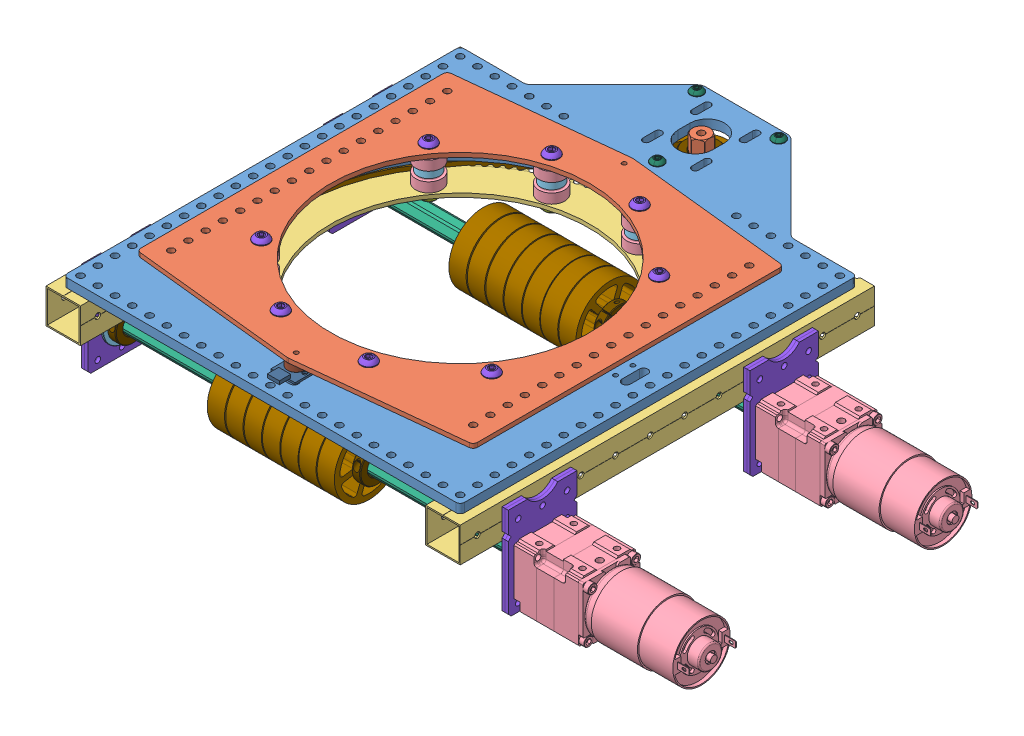
SolidWorks assembly WCP-0280 Rev1 - GreyT Turret, configuration Default. Lengths in mm.
Overall size (454.1 179.88 363.61).
150 component instances, 27 part files, 4 mates.
Components (placement in the parent):
- WCP-0280-001 Rev1-1: WCP-0280-001 Rev1 [Default] at origin size (292.1 6.6 356.64)
- spinner_tray_+_sprocket^WCP-0280 Rev1 - GreyT Turret-1: spinner_tray_+_sprocket^WCP-0280 Rev1 - GreyT Turret [Default] at origin size (248.55 39.23 334.09)
  - WCP-0280-002 Rev1-1: WCP-0280-002 Rev1 [Default] at (0 12.9476 0) size (247.65 3.17 254)
  - WCP-0280-004 Rev1-1: WCP-0280-004 Rev1 [Default] at (0 -14.1605 0) size (246.3 3.25 246.3)
  - bearing_assembly^spinner_tray_+_sprocket-1: bearing_assembly^spinner_tray_+_sprocket [Default] at (-31.5529 25.185 -41.3287) size (26.53 39.23 26.53)
    - WCP-0212_0_250_radial_bearing-1: WCP-0212_0_250_radial_bearing [Default] at (-53.2118 -18.2653 102.9139) x (-0.999427 0 0.033839) z (0 -1 0) size (19.05 19.05 7.14)
    - WCP-0212_0_250_radial_bearing-2: WCP-0212_0_250_radial_bearing [Default] at (-53.2118 -32.1147 102.9139) x (-0.572891 0 0.819632) z (0 1 0) size (19.05 19.05 7.14)
    - WCP-0041_0_250_radial_bearing-1: WCP-0041_0_250_radial_bearing [Default] at (-53.2118 -25.19 102.9139) x (-0.872331 0 0.488916) z (0 -1 0) size (15.88 15.88 4.98)
    - NFS-0011_0_250ID_fiber_washer_95601A310-1: NFS-0011_0_250ID_fiber_washer_95601A310 [Default] at (-53.2118 -35.6866 102.9139) x (0 -1 0) z (-0.326131 0 -0.945325) size (0.86 9.53 9.53)
    - NFS-0011_0_250ID_fiber_washer_95601A310-2: NFS-0011_0_250ID_fiber_washer_95601A310 [Default] at (-53.2118 -22.7008 102.9139) x (0 1 0) z (-0.943269 0 0.332029) size (0.86 9.53 9.53)
    - NFS-0011_0_250ID_fiber_washer_95601A310-3: NFS-0011_0_250ID_fiber_washer_95601A310 [Default] at (-53.2118 -28.5428 102.9139) x (0 1 0) z (-0.160822 0 -0.986983) size (0.86 9.53 9.53)
    - NFS-0011_0_250ID_fiber_washer_95601A310-4: NFS-0011_0_250ID_fiber_washer_95601A310 [Default] at (-53.2118 -14.6935 102.9139) x (0 1 0) z (-0.168532 0 -0.985696) size (0.86 9.53 9.53)
    - NFS-0024_250-20_thin_locknut_90566A029-1: NFS-0024_250-20_thin_locknut_90566A029 [Default] at (-53.2118 -39.3502 102.9139) x (0.28034 0 -0.959901) z (-0.959901 0 -0.28034) size (11.11 5.35 12.83)
    - NFS-0057_SHCS_250-20_1_375L_91255A526-1: NFS-0057_SHCS_250-20_1_375L_91255A526 [Default] at (-53.2118 -7.2971 102.9139) x (0.67695 0 0.736029) z (0 1 0) size (11.17 11.22 39.23)
  - WCP-0280-005 Rev1-1: WCP-0280-005 Rev1 [Default] at (0 -12.7603 -88.6925) size (248.55 9 320.83)
  - hall_effect_board_WCP-0971-1: hall_effect_board_WCP-0971 [Default] at (-8.89 3.302 116.459) x (-1 0 0) z (0 1 0) size (17.78 21.08 5.08)
  - hall_effect_magnet_WCP-0030-1: hall_effect_magnet_WCP-0030 [Default] at (0 8.8602 120.65) x (0.543179 0 0.839617) z (-0.839617 0 0.543179) size (12.7 5 12.7)
  - bearing_assembly^spinner_tray_+_sprocket-2: bearing_assembly^spinner_tray_+_sprocket [Default] at (-51.901 25.185 -172.6831) x (0.982082 0 -0.188455) z (0.188455 0 0.982082) size (26.53 39.23 26.53)
    - WCP-0212_0_250_radial_bearing-1: WCP-0212_0_250_radial_bearing [Default] at (-53.2118 -18.2653 102.9139) x (-0.999427 0 0.033839) z (0 -1 0) size (19.05 19.05 7.14)
    - WCP-0212_0_250_radial_bearing-2: WCP-0212_0_250_radial_bearing [Default] at (-53.2118 -32.1147 102.9139) x (-0.572891 0 0.819632) z (0 1 0) size (19.05 19.05 7.14)
    - WCP-0041_0_250_radial_bearing-1: WCP-0041_0_250_radial_bearing [Default] at (-53.2118 -25.19 102.9139) x (-0.872331 0 0.488916) z (0 -1 0) size (15.88 15.88 4.98)
    - NFS-0011_0_250ID_fiber_washer_95601A310-1: NFS-0011_0_250ID_fiber_washer_95601A310 [Default] at (-53.2118 -35.6866 102.9139) x (0 -1 0) z (-0.326131 0 -0.945325) size (0.86 9.53 9.53)
    - NFS-0011_0_250ID_fiber_washer_95601A310-2: NFS-0011_0_250ID_fiber_washer_95601A310 [Default] at (-53.2118 -22.7008 102.9139) x (0 1 0) z (-0.943269 0 0.332029) size (0.86 9.53 9.53)
    - NFS-0011_0_250ID_fiber_washer_95601A310-3: NFS-0011_0_250ID_fiber_washer_95601A310 [Default] at (-53.2118 -28.5428 102.9139) x (0 1 0) z (-0.160822 0 -0.986983) size (0.86 9.53 9.53)
    - NFS-0011_0_250ID_fiber_washer_95601A310-4: NFS-0011_0_250ID_fiber_washer_95601A310 [Default] at (-53.2118 -14.6935 102.9139) x (0 1 0) z (-0.168532 0 -0.985696) size (0.86 9.53 9.53)
    - NFS-0024_250-20_thin_locknut_90566A029-1: NFS-0024_250-20_thin_locknut_90566A029 [Default] at (-53.2118 -39.3502 102.9139) x (0.28034 0 -0.959901) z (-0.959901 0 -0.28034) size (11.11 5.35 12.83)
    - NFS-0057_SHCS_250-20_1_375L_91255A526-1: NFS-0057_SHCS_250-20_1_375L_91255A526 [Default] at (-53.2118 -7.2971 102.9139) x (0.67695 0 0.736029) z (0 1 0) size (11.17 11.22 39.23)
  - bearing_assembly^spinner_tray_+_sprocket-3: bearing_assembly^spinner_tray_+_sprocket [Default] at (-24.2359 25.185 -215.2172) x (0.918365 0 -0.395734) z (0.395734 0 0.918365) size (26.53 39.23 26.53)
    - WCP-0212_0_250_radial_bearing-1: WCP-0212_0_250_radial_bearing [Default] at (-53.2118 -18.2653 102.9139) x (-0.999427 0 0.033839) z (0 -1 0) size (19.05 19.05 7.14)
    - WCP-0212_0_250_radial_bearing-2: WCP-0212_0_250_radial_bearing [Default] at (-53.2118 -32.1147 102.9139) x (-0.572891 0 0.819632) z (0 1 0) size (19.05 19.05 7.14)
    - WCP-0041_0_250_radial_bearing-1: WCP-0041_0_250_radial_bearing [Default] at (-53.2118 -25.19 102.9139) x (-0.872331 0 0.488916) z (0 -1 0) size (15.88 15.88 4.98)
    - NFS-0011_0_250ID_fiber_washer_95601A310-1: NFS-0011_0_250ID_fiber_washer_95601A310 [Default] at (-53.2118 -35.6866 102.9139) x (0 -1 0) z (-0.326131 0 -0.945325) size (0.86 9.53 9.53)
    - NFS-0011_0_250ID_fiber_washer_95601A310-2: NFS-0011_0_250ID_fiber_washer_95601A310 [Default] at (-53.2118 -22.7008 102.9139) x (0 1 0) z (-0.943269 0 0.332029) size (0.86 9.53 9.53)
    - NFS-0011_0_250ID_fiber_washer_95601A310-3: NFS-0011_0_250ID_fiber_washer_95601A310 [Default] at (-53.2118 -28.5428 102.9139) x (0 1 0) z (-0.160822 0 -0.986983) size (0.86 9.53 9.53)
    - NFS-0011_0_250ID_fiber_washer_95601A310-4: NFS-0011_0_250ID_fiber_washer_95601A310 [Default] at (-53.2118 -14.6935 102.9139) x (0 1 0) z (-0.168532 0 -0.985696) size (0.86 9.53 9.53)
    - NFS-0024_250-20_thin_locknut_90566A029-1: NFS-0024_250-20_thin_locknut_90566A029 [Default] at (-53.2118 -39.3502 102.9139) x (0.28034 0 -0.959901) z (-0.959901 0 -0.28034) size (11.11 5.35 12.83)
    - NFS-0057_SHCS_250-20_1_375L_91255A526-1: NFS-0057_SHCS_250-20_1_375L_91255A526 [Default] at (-53.2118 -7.2971 102.9139) x (0.67695 0 0.736029) z (0 1 0) size (11.17 11.22 39.23)
  - bearing_assembly^spinner_tray_+_sprocket-4: bearing_assembly^spinner_tray_+_sprocket [Default] at (13.1984 25.185 -213.9052) x (0.8 0 -0.6) z (0.6 0 0.8) size (26.53 39.23 26.53)
    - WCP-0212_0_250_radial_bearing-1: WCP-0212_0_250_radial_bearing [Default] at (-53.2118 -18.2653 102.9139) x (-0.999427 0 0.033839) z (0 -1 0) size (19.05 19.05 7.14)
    - WCP-0212_0_250_radial_bearing-2: WCP-0212_0_250_radial_bearing [Default] at (-53.2118 -32.1147 102.9139) x (-0.572891 0 0.819632) z (0 1 0) size (19.05 19.05 7.14)
    - WCP-0041_0_250_radial_bearing-1: WCP-0041_0_250_radial_bearing [Default] at (-53.2118 -25.19 102.9139) x (-0.872331 0 0.488916) z (0 -1 0) size (15.88 15.88 4.98)
    - NFS-0011_0_250ID_fiber_washer_95601A310-1: NFS-0011_0_250ID_fiber_washer_95601A310 [Default] at (-53.2118 -35.6866 102.9139) x (0 -1 0) z (-0.326131 0 -0.945325) size (0.86 9.53 9.53)
    - NFS-0011_0_250ID_fiber_washer_95601A310-2: NFS-0011_0_250ID_fiber_washer_95601A310 [Default] at (-53.2118 -22.7008 102.9139) x (0 1 0) z (-0.943269 0 0.332029) size (0.86 9.53 9.53)
    - NFS-0011_0_250ID_fiber_washer_95601A310-3: NFS-0011_0_250ID_fiber_washer_95601A310 [Default] at (-53.2118 -28.5428 102.9139) x (0 1 0) z (-0.160822 0 -0.986983) size (0.86 9.53 9.53)
    - NFS-0011_0_250ID_fiber_washer_95601A310-4: NFS-0011_0_250ID_fiber_washer_95601A310 [Default] at (-53.2118 -14.6935 102.9139) x (0 1 0) z (-0.168532 0 -0.985696) size (0.86 9.53 9.53)
    - NFS-0024_250-20_thin_locknut_90566A029-1: NFS-0024_250-20_thin_locknut_90566A029 [Default] at (-53.2118 -39.3502 102.9139) x (0.28034 0 -0.959901) z (-0.959901 0 -0.28034) size (11.11 5.35 12.83)
    - NFS-0057_SHCS_250-20_1_375L_91255A526-1: NFS-0057_SHCS_250-20_1_375L_91255A526 [Default] at (-53.2118 -7.2971 102.9139) x (0.67695 0 0.736029) z (0 1 0) size (11.17 11.22 39.23)
  - bearing_assembly^spinner_tray_+_sprocket-5: bearing_assembly^spinner_tray_+_sprocket [Default] at (38.8565 25.185 -167.9581) x (0.63358 0 -0.773678) z (0.773678 0 0.63358) size (26.53 39.23 26.53)
    - WCP-0212_0_250_radial_bearing-1: WCP-0212_0_250_radial_bearing [Default] at (-53.2118 -18.2653 102.9139) x (-0.999427 0 0.033839) z (0 -1 0) size (19.05 19.05 7.14)
    - WCP-0212_0_250_radial_bearing-2: WCP-0212_0_250_radial_bearing [Default] at (-53.2118 -32.1147 102.9139) x (-0.572891 0 0.819632) z (0 1 0) size (19.05 19.05 7.14)
    - WCP-0041_0_250_radial_bearing-1: WCP-0041_0_250_radial_bearing [Default] at (-53.2118 -25.19 102.9139) x (-0.872331 0 0.488916) z (0 -1 0) size (15.88 15.88 4.98)
    - NFS-0011_0_250ID_fiber_washer_95601A310-1: NFS-0011_0_250ID_fiber_washer_95601A310 [Default] at (-53.2118 -35.6866 102.9139) x (0 -1 0) z (-0.326131 0 -0.945325) size (0.86 9.53 9.53)
    - NFS-0011_0_250ID_fiber_washer_95601A310-2: NFS-0011_0_250ID_fiber_washer_95601A310 [Default] at (-53.2118 -22.7008 102.9139) x (0 1 0) z (-0.943269 0 0.332029) size (0.86 9.53 9.53)
    - NFS-0011_0_250ID_fiber_washer_95601A310-3: NFS-0011_0_250ID_fiber_washer_95601A310 [Default] at (-53.2118 -28.5428 102.9139) x (0 1 0) z (-0.160822 0 -0.986983) size (0.86 9.53 9.53)
    - NFS-0011_0_250ID_fiber_washer_95601A310-4: NFS-0011_0_250ID_fiber_washer_95601A310 [Default] at (-53.2118 -14.6935 102.9139) x (0 1 0) z (-0.168532 0 -0.985696) size (0.86 9.53 9.53)
    - NFS-0024_250-20_thin_locknut_90566A029-1: NFS-0024_250-20_thin_locknut_90566A029 [Default] at (-53.2118 -39.3502 102.9139) x (0.28034 0 -0.959901) z (-0.959901 0 -0.28034) size (11.11 5.35 12.83)
    - NFS-0057_SHCS_250-20_1_375L_91255A526-1: NFS-0057_SHCS_250-20_1_375L_91255A526 [Default] at (-53.2118 -7.2971 102.9139) x (0.67695 0 0.736029) z (0 1 0) size (11.17 11.22 39.23)
  - bearing_assembly^spinner_tray_+_sprocket-6: bearing_assembly^spinner_tray_+_sprocket [Default] at (16.1385 25.185 -31.7594) x (0.443629 0 -0.896211) z (0.896211 0 0.443629) size (26.53 39.23 26.53)
    - WCP-0212_0_250_radial_bearing-1: WCP-0212_0_250_radial_bearing [Default] at (-53.2118 -18.2653 102.9139) x (-0.999427 0 0.033839) z (0 -1 0) size (19.05 19.05 7.14)
    - WCP-0212_0_250_radial_bearing-2: WCP-0212_0_250_radial_bearing [Default] at (-53.2118 -32.1147 102.9139) x (-0.572891 0 0.819632) z (0 1 0) size (19.05 19.05 7.14)
    - WCP-0041_0_250_radial_bearing-1: WCP-0041_0_250_radial_bearing [Default] at (-53.2118 -25.19 102.9139) x (-0.872331 0 0.488916) z (0 -1 0) size (15.88 15.88 4.98)
    - NFS-0011_0_250ID_fiber_washer_95601A310-1: NFS-0011_0_250ID_fiber_washer_95601A310 [Default] at (-53.2118 -35.6866 102.9139) x (0 -1 0) z (-0.326131 0 -0.945325) size (0.86 9.53 9.53)
    - NFS-0011_0_250ID_fiber_washer_95601A310-2: NFS-0011_0_250ID_fiber_washer_95601A310 [Default] at (-53.2118 -22.7008 102.9139) x (0 1 0) z (-0.943269 0 0.332029) size (0.86 9.53 9.53)
    - NFS-0011_0_250ID_fiber_washer_95601A310-3: NFS-0011_0_250ID_fiber_washer_95601A310 [Default] at (-53.2118 -28.5428 102.9139) x (0 1 0) z (-0.160822 0 -0.986983) size (0.86 9.53 9.53)
    - NFS-0011_0_250ID_fiber_washer_95601A310-4: NFS-0011_0_250ID_fiber_washer_95601A310 [Default] at (-53.2118 -14.6935 102.9139) x (0 1 0) z (-0.168532 0 -0.985696) size (0.86 9.53 9.53)
    - NFS-0024_250-20_thin_locknut_90566A029-1: NFS-0024_250-20_thin_locknut_90566A029 [Default] at (-53.2118 -39.3502 102.9139) x (0.28034 0 -0.959901) z (-0.959901 0 -0.28034) size (11.11 5.35 12.83)
    - NFS-0057_SHCS_250-20_1_375L_91255A526-1: NFS-0057_SHCS_250-20_1_375L_91255A526 [Default] at (-53.2118 -7.2971 102.9139) x (0.67695 0 0.736029) z (0 1 0) size (11.17 11.22 39.23)
  - bearing_assembly^spinner_tray_+_sprocket-7: bearing_assembly^spinner_tray_+_sprocket [Default] at (-52.9007 25.185 21.2222) x (0.263225 0 -0.964735) z (0.964735 0 0.263225) size (26.53 39.23 26.53)
    - WCP-0212_0_250_radial_bearing-1: WCP-0212_0_250_radial_bearing [Default] at (-53.2118 -18.2653 102.9139) x (-0.999427 0 0.033839) z (0 -1 0) size (19.05 19.05 7.14)
    - WCP-0212_0_250_radial_bearing-2: WCP-0212_0_250_radial_bearing [Default] at (-53.2118 -32.1147 102.9139) x (-0.572891 0 0.819632) z (0 1 0) size (19.05 19.05 7.14)
    - WCP-0041_0_250_radial_bearing-1: WCP-0041_0_250_radial_bearing [Default] at (-53.2118 -25.19 102.9139) x (-0.872331 0 0.488916) z (0 -1 0) size (15.88 15.88 4.98)
    - NFS-0011_0_250ID_fiber_washer_95601A310-1: NFS-0011_0_250ID_fiber_washer_95601A310 [Default] at (-53.2118 -35.6866 102.9139) x (0 -1 0) z (-0.326131 0 -0.945325) size (0.86 9.53 9.53)
    - NFS-0011_0_250ID_fiber_washer_95601A310-2: NFS-0011_0_250ID_fiber_washer_95601A310 [Default] at (-53.2118 -22.7008 102.9139) x (0 1 0) z (-0.943269 0 0.332029) size (0.86 9.53 9.53)
    - NFS-0011_0_250ID_fiber_washer_95601A310-3: NFS-0011_0_250ID_fiber_washer_95601A310 [Default] at (-53.2118 -28.5428 102.9139) x (0 1 0) z (-0.160822 0 -0.986983) size (0.86 9.53 9.53)
    - NFS-0011_0_250ID_fiber_washer_95601A310-4: NFS-0011_0_250ID_fiber_washer_95601A310 [Default] at (-53.2118 -14.6935 102.9139) x (0 1 0) z (-0.168532 0 -0.985696) size (0.86 9.53 9.53)
    - NFS-0024_250-20_thin_locknut_90566A029-1: NFS-0024_250-20_thin_locknut_90566A029 [Default] at (-53.2118 -39.3502 102.9139) x (0.28034 0 -0.959901) z (-0.959901 0 -0.28034) size (11.11 5.35 12.83)
    - NFS-0057_SHCS_250-20_1_375L_91255A526-1: NFS-0057_SHCS_250-20_1_375L_91255A526 [Default] at (-53.2118 -7.2971 102.9139) x (0.67695 0 0.736029) z (0 1 0) size (11.17 11.22 39.23)
  - bearing_assembly^spinner_tray_+_sprocket-8: bearing_assembly^spinner_tray_+_sprocket [Default] at (-128.1504 25.185 34.4528) x (0.120178 0 -0.992752) z (0.992752 0 0.120178) size (26.53 39.23 26.53)
    - WCP-0212_0_250_radial_bearing-1: WCP-0212_0_250_radial_bearing [Default] at (-53.2118 -18.2653 102.9139) x (-0.999427 0 0.033839) z (0 -1 0) size (19.05 19.05 7.14)
    - WCP-0212_0_250_radial_bearing-2: WCP-0212_0_250_radial_bearing [Default] at (-53.2118 -32.1147 102.9139) x (-0.572891 0 0.819632) z (0 1 0) size (19.05 19.05 7.14)
    - WCP-0041_0_250_radial_bearing-1: WCP-0041_0_250_radial_bearing [Default] at (-53.2118 -25.19 102.9139) x (-0.872331 0 0.488916) z (0 -1 0) size (15.88 15.88 4.98)
    - NFS-0011_0_250ID_fiber_washer_95601A310-1: NFS-0011_0_250ID_fiber_washer_95601A310 [Default] at (-53.2118 -35.6866 102.9139) x (0 -1 0) z (-0.326131 0 -0.945325) size (0.86 9.53 9.53)
    - NFS-0011_0_250ID_fiber_washer_95601A310-2: NFS-0011_0_250ID_fiber_washer_95601A310 [Default] at (-53.2118 -22.7008 102.9139) x (0 1 0) z (-0.943269 0 0.332029) size (0.86 9.53 9.53)
    - NFS-0011_0_250ID_fiber_washer_95601A310-3: NFS-0011_0_250ID_fiber_washer_95601A310 [Default] at (-53.2118 -28.5428 102.9139) x (0 1 0) z (-0.160822 0 -0.986983) size (0.86 9.53 9.53)
    - NFS-0011_0_250ID_fiber_washer_95601A310-4: NFS-0011_0_250ID_fiber_washer_95601A310 [Default] at (-53.2118 -14.6935 102.9139) x (0 1 0) z (-0.168532 0 -0.985696) size (0.86 9.53 9.53)
    - NFS-0024_250-20_thin_locknut_90566A029-1: NFS-0024_250-20_thin_locknut_90566A029 [Default] at (-53.2118 -39.3502 102.9139) x (0.28034 0 -0.959901) z (-0.959901 0 -0.28034) size (11.11 5.35 12.83)
    - NFS-0057_SHCS_250-20_1_375L_91255A526-1: NFS-0057_SHCS_250-20_1_375L_91255A526 [Default] at (-53.2118 -7.2971 102.9139) x (0.67695 0 0.736029) z (0 1 0) size (11.17 11.22 39.23)
- turret_swivel_motor_assembly^WCP-0280 Rev1 - GreyT Turret-1: turret_swivel_motor_assembly^WCP-0280 Rev1 - GreyT Turret [Default] at origin size (73.41 167.54 80.86)
  - WCP-0280-003 Rev1-1: WCP-0280-003 Rev1 [Default] at (0 -33.4645 -177.3845) size (73.03 3.17 73.44)
  - wcd_cam_217-3431-1: wcd_cam_217-3431 [Default] at (-2.1071 -41.402 -145.7696) x (0.727312 0 -0.686307) z (0 -1 0) size (22.69 21.26 12.7)
  - WCP-0226 Rev1-1: WCP-0226 Rev1 [Default] at (30.1625 -17.5895 -204.235) x (0 1 0) z (-0.493388 0 0.869809) size (28.57 9.5 9.5)
  - WCP-0226 Rev1-2: WCP-0226 Rev1 [Default] at (0 -17.5895 -145.0815) x (0 1 0) z (-0.104761 0 0.994497) size (28.57 9.5 9.5)
  - WCP-0226 Rev1-3: WCP-0226 Rev1 [Default] at (-30.1625 -17.5895 -204.235) x (0 1 0) z (-0.104761 0 0.994497) size (28.57 9.5 9.5)
  - WCP-0258 Rev1-1: WCP-0258 Rev1 [Default] at (0 5.8674 -145.0815) x (0.945142 0 -0.32666) z (0 1 0) size (9.2 9.23 49.52)
  - WCP-0258 Rev1-2: WCP-0258 Rev1 [Default] at (-30.1625 5.8674 -204.235) x (0.945142 0 -0.32666) z (0 1 0) size (9.2 9.23 49.52)
  - WCP-0258 Rev1-3: WCP-0258 Rev1 [Default] at (30.1625 5.8674 -204.235) x (0.945142 0 -0.32666) z (0 1 0) size (9.2 9.23 49.52)
  - NFS-0010_#10-32_thin_locknut_Default_As Machined_-1: NFS-0010_#10-32_thin_locknut_Default_As Machined_ [Default] at (-30.1625 -35.052 -204.235) x (0.910739 0 -0.412983) z (-0.412983 0 -0.910739) size (9.53 4.37 11)
  - NFS-0010_#10-32_thin_locknut_Default_As Machined_-2: NFS-0010_#10-32_thin_locknut_Default_As Machined_ [Default] at (30.1625 -35.052 -204.235) x (-0.933743 0 -0.357945) z (-0.357945 0 0.933743) size (9.53 4.37 11)
  - WCP-0253 Rev1-1: WCP-0253 Rev1 [Default] at (17.9605 -29.3116 -159.4245) x (0.553393 0 -0.83292) z (0 1 0) size (9.24 9.28 15.9)
  - WCP-0253 Rev1-2: WCP-0253 Rev1 [Default] at (-17.9605 -29.3116 -195.3456) x (-0.735473 0 -0.677555) z (0 1 0) size (9.24 9.28 15.9)
  - 217-2737_500_hex_collar-1: 217-2737_500_hex_collar [Default] at (0 -23.7141 -177.3851) x (0.975283 0 0.220959) z (0 1 0) size (25.39 25.4 7.82)
  - 217-2737_500_hex_collar-2: 217-2737_500_hex_collar [Default] at (0 -8.1883 -177.3851) x (0.855545 0 0.517728) z (0 -1 0) size (25.39 25.4 7.82)
  - 217-2642_16T_500_hex-1: 217-2642_16T_500_hex [Default] at (0 -14.1573 -177.3851) x (0.551766 0 -0.833999) z (0 1 0) size (35.21 35.21 9.18)
  - v2_versa_planetary_1_stage-1: v2_versa_planetary_1_stage [Default] at (22.225 -51.677 -177.3851) x (0 1 0) z (0 0 1) size (166.6 44.45 44.3)
- 1x1_tube_stock_WCP-0280-006 Rev1-1: 1x1_tube_stock_WCP-0280-006 Rev1 [Default] at (139.7 -16.002 -596.9) size (25.4 25.4 304.8)
- 1x1_tube_stock_WCP-0280-006 Rev1-2: 1x1_tube_stock_WCP-0280-006 Rev1 [Default] at (-139.7 -16.002 -596.9) size (25.4 25.4 304.8)
- pre-roller_assembly-1: pre-roller_assembly [Default] at origin size (454.1 80.43 71.81)
  - v2_versa_planetary_1_stage_no_output-1: v2_versa_planetary_1_stage_no_output [Default] at (173.597 -73.6827 96.3395) x (-1 0 0) z (0 0 -1) size (126.03 44.45 44.3)
  - 217-4006_0_500_flanged_thunderhex_bearing-1: 217-4006_0_500_flanged_thunderhex_bearing [Default] at (-154.7812 -51.4577 96.3395) x (0 -0.481649 -0.876364) z (1 0 0) size (31.12 31.12 7.94)
  - WCP-0280-007 Rev1-1: WCP-0280-007 Rev1 [Default] at (-12.3532 -51.4577 96.3395) x (1 0 0) z (0 -0.918939 0.3944) size (317.5 12.7 13.75)
  - WCP-0253 Rev1-1: WCP-0253 Rev1 [Default] at (149.8346 -69.4182 78.379) x (0 -0.851264 -0.524738) z (-1 0 0) size (9.24 9.28 15.9)
  - WCP-0253 Rev1-2: WCP-0253 Rev1 [Default] at (149.8346 -33.4972 114.3) x (0 0.557595 -0.830113) z (-1 0 0) size (9.24 9.28 15.9)
  - 217-2737_500_hex_collar-1: 217-2737_500_hex_collar [Default] at (-161.925 -51.4577 96.3395) x (0 0.97196 0.235146) z (1 0 0) size (25.39 25.4 7.82)
  - 217-2737_500_hex_collar-2: 217-2737_500_hex_collar [Default] at (-147.6375 -51.4577 96.3395) x (0 0.799523 0.600635) z (-1 0 0) size (25.39 25.4 7.82)
  - Universal_Female_Output_Shaft_1_2_Hex-1: Universal_Female_Output_Shaft_1_2_Hex [Default] at (166.1492 -51.4577 96.3395) x (0 0.997742 0.067166) z (-1 0 0) size (21.37 20 42.62)
  - 217-4183_VersaFrame_Face_Bearing_Mount-1: 217-4183_VersaFrame_Face_Bearing_Mount [Default] at (154.686 -24.7496 96.3395) x (0 -1 0) z (1 0 0) size (68.49 50.55 2.29)
  - 217-4183_VersaFrame_Face_Bearing_Mount-2: 217-4183_VersaFrame_Face_Bearing_Mount [Default] at (152.4 -24.7496 96.3395) x (0 -1 0) z (1 0 0) size (68.49 50.55 2.29)
  - 217-4183_VersaFrame_Face_Bearing_Mount-3: 217-4183_VersaFrame_Face_Bearing_Mount [Default] at (-154.686 -24.7496 96.3395) x (0 -1 0) z (1 0 0) size (68.49 50.55 2.29)
  - 217-4183_VersaFrame_Face_Bearing_Mount-4: 217-4183_VersaFrame_Face_Bearing_Mount [Default] at (-156.972 -24.7496 96.3395) x (0 -1 0) z (1 0 0) size (68.49 50.55 2.29)
  - 2_OD_Straight_Flex_Wheel_217-6446-1: 2_OD_Straight_Flex_Wheel_217-6446 [Default] at (9.3117 -51.4577 96.3395) x (0 0.610406 -0.792088) z (0 0.792088 0.610406) size (50.8 12.7 50.8)
  - 2_OD_Straight_Flex_Wheel_217-6446-2: 2_OD_Straight_Flex_Wheel_217-6446 [Default] at (-58.0571 -51.4577 96.3395) x (0 0.249738 -0.968314) z (0 0.968314 0.249738) size (50.8 12.7 50.8)
  - 2_OD_Straight_Flex_Wheel_217-6446-3: 2_OD_Straight_Flex_Wheel_217-6446 [Default] at (-3.9428 -51.4577 96.3395) x (0 -0.070457 -0.997515) z (0 0.997515 -0.070457) size (50.8 12.7 50.8)
  - 217-2737_500_hex_collar-3: 217-2737_500_hex_collar [Default] at (32.3405 -51.4577 96.3395) x (0 0.832718 0.553698) z (-1 0 0) size (25.39 25.4 7.82)
  - 217-2737_500_hex_collar-4: 217-2737_500_hex_collar [Default] at (-68.0772 -51.4577 96.3395) x (0 0.724871 0.688884) z (-1 0 0) size (25.39 25.4 7.82)
  - 2_OD_Straight_Flex_Wheel_217-6446-4: 2_OD_Straight_Flex_Wheel_217-6446 [Default] at (-30.9117 -51.4577 96.3395) x (0 0.410417 -0.911898) z (0 0.911898 0.410417) size (50.8 12.7 50.8)
  - 2_OD_Straight_Flex_Wheel_217-6446-5: 2_OD_Straight_Flex_Wheel_217-6446 [Default] at (-17.4177 -51.4577 96.3395) x (0 0.496878 -0.86782) z (0 0.86782 0.496878) size (50.8 12.7 50.8)
  - 2_OD_Straight_Flex_Wheel_217-6446-6: 2_OD_Straight_Flex_Wheel_217-6446 [Default] at (-44.4634 -51.4577 96.3395) x (0 0.687316 -0.726359) z (0 0.726359 0.687316) size (50.8 12.7 50.8)
  - 2_OD_Straight_Flex_Wheel_217-6446-7: 2_OD_Straight_Flex_Wheel_217-6446 [Default] at (22.7808 -51.4577 96.3395) x (0 0.629554 -0.776957) z (0 0.776957 0.629554) size (50.8 12.7 50.8)
- pre-roller_assembly-2: pre-roller_assembly [Default] at (0 0 -177.8) size (454.1 80.43 71.81)
  - v2_versa_planetary_1_stage_no_output-1: v2_versa_planetary_1_stage_no_output [Default] at (173.597 -73.6827 96.3395) x (-1 0 0) z (0 0 -1) size (126.03 44.45 44.3)
  - 217-4006_0_500_flanged_thunderhex_bearing-1: 217-4006_0_500_flanged_thunderhex_bearing [Default] at (-154.7812 -51.4577 96.3395) x (0 -0.481649 -0.876364) z (1 0 0) size (31.12 31.12 7.94)
  - WCP-0280-007 Rev1-1: WCP-0280-007 Rev1 [Default] at (-12.3532 -51.4577 96.3395) x (1 0 0) z (0 -0.918939 0.3944) size (317.5 12.7 13.75)
  - WCP-0253 Rev1-1: WCP-0253 Rev1 [Default] at (149.8346 -69.4182 78.379) x (0 -0.851264 -0.524738) z (-1 0 0) size (9.24 9.28 15.9)
  - WCP-0253 Rev1-2: WCP-0253 Rev1 [Default] at (149.8346 -33.4972 114.3) x (0 0.557595 -0.830113) z (-1 0 0) size (9.24 9.28 15.9)
  - 217-2737_500_hex_collar-1: 217-2737_500_hex_collar [Default] at (-161.925 -51.4577 96.3395) x (0 0.97196 0.235146) z (1 0 0) size (25.39 25.4 7.82)
  - 217-2737_500_hex_collar-2: 217-2737_500_hex_collar [Default] at (-147.6375 -51.4577 96.3395) x (0 0.799523 0.600635) z (-1 0 0) size (25.39 25.4 7.82)
  - Universal_Female_Output_Shaft_1_2_Hex-1: Universal_Female_Output_Shaft_1_2_Hex [Default] at (166.1492 -51.4577 96.3395) x (0 0.997742 0.067166) z (-1 0 0) size (21.37 20 42.62)
  - 217-4183_VersaFrame_Face_Bearing_Mount-1: 217-4183_VersaFrame_Face_Bearing_Mount [Default] at (154.686 -24.7496 96.3395) x (0 -1 0) z (1 0 0) size (68.49 50.55 2.29)
  - 217-4183_VersaFrame_Face_Bearing_Mount-2: 217-4183_VersaFrame_Face_Bearing_Mount [Default] at (152.4 -24.7496 96.3395) x (0 -1 0) z (1 0 0) size (68.49 50.55 2.29)
  - 217-4183_VersaFrame_Face_Bearing_Mount-3: 217-4183_VersaFrame_Face_Bearing_Mount [Default] at (-154.686 -24.7496 96.3395) x (0 -1 0) z (1 0 0) size (68.49 50.55 2.29)
  - 217-4183_VersaFrame_Face_Bearing_Mount-4: 217-4183_VersaFrame_Face_Bearing_Mount [Default] at (-156.972 -24.7496 96.3395) x (0 -1 0) z (1 0 0) size (68.49 50.55 2.29)
  - 2_OD_Straight_Flex_Wheel_217-6446-1: 2_OD_Straight_Flex_Wheel_217-6446 [Default] at (9.3117 -51.4577 96.3395) x (0 0.610406 -0.792088) z (0 0.792088 0.610406) size (50.8 12.7 50.8)
  - 2_OD_Straight_Flex_Wheel_217-6446-2: 2_OD_Straight_Flex_Wheel_217-6446 [Default] at (-58.0571 -51.4577 96.3395) x (0 0.249738 -0.968314) z (0 0.968314 0.249738) size (50.8 12.7 50.8)
  - 2_OD_Straight_Flex_Wheel_217-6446-3: 2_OD_Straight_Flex_Wheel_217-6446 [Default] at (-3.9428 -51.4577 96.3395) x (0 -0.070457 -0.997515) z (0 0.997515 -0.070457) size (50.8 12.7 50.8)
  - 217-2737_500_hex_collar-3: 217-2737_500_hex_collar [Default] at (32.3405 -51.4577 96.3395) x (0 0.832718 0.553698) z (-1 0 0) size (25.39 25.4 7.82)
  - 217-2737_500_hex_collar-4: 217-2737_500_hex_collar [Default] at (-68.0772 -51.4577 96.3395) x (0 0.724871 0.688884) z (-1 0 0) size (25.39 25.4 7.82)
  - 2_OD_Straight_Flex_Wheel_217-6446-4: 2_OD_Straight_Flex_Wheel_217-6446 [Default] at (-30.9117 -51.4577 96.3395) x (0 0.410417 -0.911898) z (0 0.911898 0.410417) size (50.8 12.7 50.8)
  - 2_OD_Straight_Flex_Wheel_217-6446-5: 2_OD_Straight_Flex_Wheel_217-6446 [Default] at (-17.4177 -51.4577 96.3395) x (0 0.496878 -0.86782) z (0 0.86782 0.496878) size (50.8 12.7 50.8)
  - 2_OD_Straight_Flex_Wheel_217-6446-6: 2_OD_Straight_Flex_Wheel_217-6446 [Default] at (-44.4634 -51.4577 96.3395) x (0 0.687316 -0.726359) z (0 0.726359 0.687316) size (50.8 12.7 50.8)
  - 2_OD_Straight_Flex_Wheel_217-6446-7: 2_OD_Straight_Flex_Wheel_217-6446 [Default] at (22.7808 -51.4577 96.3395) x (0 0.629554 -0.776957) z (0 0.776957 0.629554) size (50.8 12.7 50.8)
Mates (geometry in assembly coordinates):
- Coincident75: coincident aligned: circle of WCP-0280-006 Rev1-2; circle of Assem2^WCP-0280 Rev1 - GreyT Turret-2/217-4183_VersaFrame_Face_Bearing_Mount-3
- Parallel5: parallel aligned: line of WCP-0280-006 Rev1-1 through (152.4 -28.702 -152.4) axis (0 1 0); line of Assem2^WCP-0280 Rev1 - GreyT Turret-2/217-4183_VersaFrame_Face_Bearing_Mount-2 through (152.4 -22.5906 -106.7335) axis (0 1 0)
- Coincident77: coincident aligned: circle of WCP-0280-006 Rev1-1; circle of Assem2^WCP-0280 Rev1 - GreyT Turret-1/217-4183_VersaFrame_Face_Bearing_Mount-2
- Parallel6: parallel aligned: line of WCP-0280-006 Rev1-2 through (-152.4 -16.0782 152.4) axis (0 -1 0); line of Assem2^WCP-0280 Rev1 - GreyT Turret-1/217-4183_VersaFrame_Face_Bearing_Mount-3 through (-152.4 -6.9315 121.6125) axis (0 -1 0)
